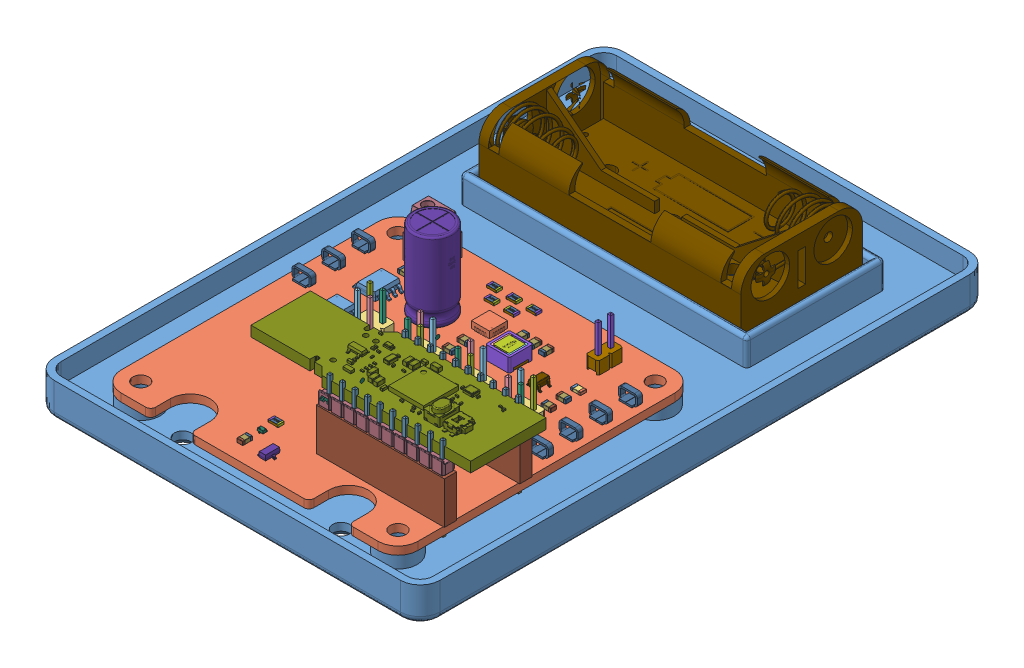
SolidWorks assembly 2228_Emetteur_Assembly, configuration Défaut. Lengths in mm.
Overall size (78 27.62 115.1).
221 component instances, 55 part files, 8 mates.
Components (placement in the parent):
- 2228_Emetteur_Bottom_wPCB-1: 2228_Emetteur_Bottom_wPCB [Défaut] at origin size (78 8.5 115.1)
- 2228_Emetteur_Top-1: 2228_Emetteur_Top [Défaut] at (0 31 0) x (-1 0 0) z (0 0 1) size (78 28 115.1) (hidden)
- 22280A_AlarmeFenetre_Emetteur.step-1: 22280A_AlarmeFenetre_Emetteur.step [Défaut] at (30 7.1063 -64.5) x (-1 0 0) z (0 1 0) size (64.32 60 20.1)
  - Board.step-1: Board.step [Défaut] at origin size (60 60 1.61)
    - Open CASCADE STEP translator 6.8 1.1.1.step-1: Open CASCADE STEP translator 6.8 1.1.1.step [Défaut] at (0 0 -1.6063) size (60 60 1.61)
  - X3.step-1: X3.step [Défaut] at origin size (5.08 5.08 11.54)
    - 61300421121.step-1: 61300421121.step [Défaut] at (31.75 25 1.27) x (0 1 0) z (1 0 0) size (5.08 11.54 5.08)
      - Open CASCADE STEP translator 6.8 1.2.1.1.step-1: Open CASCADE STEP translator 6.8 1.2.1.1.step [Défaut] at origin size (5.08 2.54 5.08)
      - Open CASCADE STEP translator 6.8 1.2.1.2.step-1: Open CASCADE STEP translator 6.8 1.2.1.2.step [Défaut] at origin size (0.64 11.54 0.64)
      - Open CASCADE STEP translator 6.8 1.2.1.3.step-1: Open CASCADE STEP translator 6.8 1.2.1.3.step [Défaut] at origin size (0.64 11.54 0.64)
      - Open CASCADE STEP translator 6.8 1.2.1.4.step-1: Open CASCADE STEP translator 6.8 1.2.1.4.step [Défaut] at origin size (0.64 11.54 0.64)
      - Open CASCADE STEP translator 6.8 1.2.1.5.step-1: Open CASCADE STEP translator 6.8 1.2.1.5.step [Défaut] at origin size (0.64 11.54 0.64)
  - X5.step-1: X5.step [Défaut] at origin size (5.08 5.08 11.54)
    - 61300421121.step-1: 61300421121.step [Défaut] at (21.59 25 1.27) x (0 1 0) z (1 0 0) size (5.08 11.54 5.08)
      - Open CASCADE STEP translator 6.8 1.2.1.1.step-1: Open CASCADE STEP translator 6.8 1.2.1.1.step [Défaut] at origin size (5.08 2.54 5.08)
      - Open CASCADE STEP translator 6.8 1.2.1.2.step-1: Open CASCADE STEP translator 6.8 1.2.1.2.step [Défaut] at origin size (0.64 11.54 0.64)
      - Open CASCADE STEP translator 6.8 1.2.1.3.step-1: Open CASCADE STEP translator 6.8 1.2.1.3.step [Défaut] at origin size (0.64 11.54 0.64)
      - Open CASCADE STEP translator 6.8 1.2.1.4.step-1: Open CASCADE STEP translator 6.8 1.2.1.4.step [Défaut] at origin size (0.64 11.54 0.64)
      - Open CASCADE STEP translator 6.8 1.2.1.5.step-1: Open CASCADE STEP translator 6.8 1.2.1.5.step [Défaut] at origin size (0.64 11.54 0.64)
  - X4.step-1: X4.step [Défaut] at origin size (5.08 5.08 11.54)
    - 61300421121.step-1: 61300421121.step [Défaut] at (10.16 26.27 1.27) x (-1 0 0) z (0 1 0) size (5.08 11.54 5.08)
      - Open CASCADE STEP translator 6.8 1.2.1.1.step-1: Open CASCADE STEP translator 6.8 1.2.1.1.step [Défaut] at origin size (5.08 2.54 5.08)
      - Open CASCADE STEP translator 6.8 1.2.1.2.step-1: Open CASCADE STEP translator 6.8 1.2.1.2.step [Défaut] at origin size (0.64 11.54 0.64)
      - Open CASCADE STEP translator 6.8 1.2.1.3.step-1: Open CASCADE STEP translator 6.8 1.2.1.3.step [Défaut] at origin size (0.64 11.54 0.64)
      - Open CASCADE STEP translator 6.8 1.2.1.4.step-1: Open CASCADE STEP translator 6.8 1.2.1.4.step [Défaut] at origin size (0.64 11.54 0.64)
      - Open CASCADE STEP translator 6.8 1.2.1.5.step-1: Open CASCADE STEP translator 6.8 1.2.1.5.step [Défaut] at origin size (0.64 11.54 0.64)
  - X2.step-1: X2.step [Défaut] at origin size (5.08 5.08 11.54)
    - 61300421121.step-1: 61300421121.step [Défaut] at (39.37 25 1.27) x (0 -1 0) z (-1 0 0) size (5.08 11.54 5.08)
      - Open CASCADE STEP translator 6.8 1.2.1.1.step-1: Open CASCADE STEP translator 6.8 1.2.1.1.step [Défaut] at origin size (5.08 2.54 5.08)
      - Open CASCADE STEP translator 6.8 1.2.1.2.step-1: Open CASCADE STEP translator 6.8 1.2.1.2.step [Défaut] at origin size (0.64 11.54 0.64)
      - Open CASCADE STEP translator 6.8 1.2.1.3.step-1: Open CASCADE STEP translator 6.8 1.2.1.3.step [Défaut] at origin size (0.64 11.54 0.64)
      - Open CASCADE STEP translator 6.8 1.2.1.4.step-1: Open CASCADE STEP translator 6.8 1.2.1.4.step [Défaut] at origin size (0.64 11.54 0.64)
      - Open CASCADE STEP translator 6.8 1.2.1.5.step-1: Open CASCADE STEP translator 6.8 1.2.1.5.step [Défaut] at origin size (0.64 11.54 0.64)
  - X1.step-1: X1.step [Défaut] at origin size (2.54 5.08 11.54)
    - STEP-61300211121-rev1.step-1: STEP-61300211121-rev1.step [Défaut] at (11.9999 6.27 1.27) x (0 -1 0) z (-1 0 0) size (5.08 11.54 2.54)
      - 6130xx11121_PIN.step-1: 6130xx11121_PIN.step [Défaut] at (-1.27 1.5 0) x (1 0 0) z (0 -1 0) size (0.64 0.64 11.54)
      - 6130xx11121_PIN.step-2: 6130xx11121_PIN.step [Défaut] at (1.27 1.5 0) x (1 0 0) z (0 -1 0) size (0.64 0.64 11.54)
      - 61300211121.step-1: 61300211121.step [Défaut] at origin size (5.08 2.54 2.54)
  - VSTOR.step-1: VSTOR.step [Défaut] at origin size (3.81 2.03 2.29)
    - keystone-PN5019.step-1: keystone-PN5019.step [Défaut] at (56.9999 22.0009 0) x (1 0 0) z (0 -1 0) size (3.81 2.29 2.03)
  - VSEC.step-1: VSEC.step [Défaut] at origin size (3.81 2.03 2.29)
    - keystone-PN5019.step-1: keystone-PN5019.step [Défaut] at (57.0001 15.9991 0) x (-1 0 0) z (0 1 0) size (3.81 2.29 2.03)
  - VMUL.step-1: VMUL.step [Défaut] at origin size (3.81 2.03 2.29)
    - keystone-PN5019.step-1: keystone-PN5019.step [Défaut] at (3.0001 21.9991 0) x (-1 0 0) z (0 1 0) size (3.81 2.29 2.03)
  - VIN.step-1: VIN.step [Défaut] at origin size (3.81 2.03 2.29)
    - keystone-PN5019.step-1: keystone-PN5019.step [Défaut] at (2.9999 10.0009 0) x (1 0 0) z (0 -1 0) size (3.81 2.29 2.03)
  - VCC.step-1: VCC.step [Défaut] at origin size (3.81 2.03 2.29)
    - keystone-PN5019.step-1: keystone-PN5019.step [Défaut] at (3.0001 27.9991 0) x (-1 0 0) z (0 1 0) size (3.81 2.29 2.03)
  - U6.step-1: U6.step [Défaut] at origin size (46.04 19.26 18.6)
    - 61301011821.step-1: 61301011821.step [Défaut] at (1.27 49.62 0) x (1 0 0) z (0 0 1) size (25.9 2.5 11.6)
      - Body.step-1: Body.step [Défaut] at origin size (25.9 2.5 8.5)
      - LeadsArray.step-1: LeadsArray.step [Défaut] at origin size (23.46 0.6 4.8)
    - 61301011821.step-2: 61301011821.step [Défaut] at (1.27 34.38 0) x (1 0 0) z (0 0 1) size (25.9 2.5 11.6)
      - Body.step-1: Body.step [Défaut] at origin size (25.9 2.5 8.5)
      - LeadsArray.step-1: LeadsArray.step [Défaut] at origin size (23.46 0.6 4.8)
    - Conn_Wurth_Elektronik_61301011121_eec.step-1: Conn_Wurth_Elektronik_61301011121_eec.step [Défaut] at (12.7 49.62 10) x (1 0 0) z (0 1 0) size (25.4 11.74 4.02)
      - Package.step-1: Package.step [Défaut] at origin size (25.4 2.54 2.54)
      - Pins.step-1: Pins.step [Défaut] at origin size (23.5 11.74 0.64)
      - Logo.step-1: Logo.step [Défaut] at (12.7 -1.27 1.27) size (5.18 4.49 4.02)
    - Conn_Wurth_Elektronik_61301011121_eec.step-2: Conn_Wurth_Elektronik_61301011121_eec.step [Défaut] at (12.7 34.38 10) x (1 0 0) z (0 1 0) size (25.4 11.74 4.02)
      - Package.step-1: Package.step [Défaut] at origin size (25.4 2.54 2.54)
      - Pins.step-1: Pins.step [Défaut] at origin size (23.5 11.74 0.64)
      - Logo.step-1: Logo.step [Défaut] at (12.7 -1.27 1.27) size (5.18 4.49 4.02)
    - 400250.step-1: 400250.step [Défaut] at (-4.318 42 13) x (1 0 0) z (0 0 1) size (46.04 15.24 4.57)
  - U5.step-1: U5.step [Défaut] at origin size (2.51 2.92 1.12)
    - 5881998176.step-1: 5881998176.step [Défaut] at (30 56 0) x (-1 0 0) z (0 1 0) size (2.51 1.12 2.92)
  - U4.step-1: U4.step [Défaut] at origin size (2.8 2.9 1.45)
    - 5881997696.step-1: 5881997696.step [Défaut] at (15 16.5 0) x (-1 0 0) z (0 1 0) size (2.8 1.45 2.9)
  - U3.step-1: U3.step [Défaut] at origin size (6.1 4.99 1.77)
    - 5882000496.step-1: 5882000496.step [Défaut] at (48 16 0) x (-1 0 0) z (0 0 1) size (6.1 4.99 1.77)
  - U2.step-1: U2.step [Défaut] at origin size (6.1 4.99 1.77)
    - 5882000496.step-1: 5882000496.step [Défaut] at (48 25 0) x (-1 0 0) z (0 0 1) size (6.1 4.99 1.77)
  - U1.step-1: U1.step [Défaut] at origin size (3.76 3.76 1.4)
    - RGR20_2P05X2P05_TEX.step-1: RGR20_2P05X2P05_TEX.step [Défaut] at (30 11.5 0) x (1 0 0) z (0 0 1) size (3.76 3.76 1.4)
  - S1.step-1: S1.step [Défaut] at origin size (23 8 1.9)
    - Anysolar_KXOB25.step-1: Anysolar_KXOB25.step [Défaut] at (30 5 -1.6063) x (1 0 0) z (0 0 -1) size (7.2 6.59 0.1)
    - Anysolar_KXOB25-0.step-1: Anysolar_KXOB25-0.step [Défaut] at (30 5 -1.6063) x (1 0 0) z (0 0 -1) size (23 8 1.8)
    - Anysolar_KXOB25-1.step-1: Anysolar_KXOB25-1.step [Défaut] at (30 5 -1.6063) x (1 0 0) z (0 0 -1) size (7.2 6.59 0.1)
    - Anysolar_KXOB25-2.step-1: Anysolar_KXOB25-2.step [Défaut] at (30 5 -1.6063) x (1 0 0) z (0 0 -1) size (7.2 6.59 0.1)
  - R6.step-1: R6.step [Défaut] at origin size (2 1.25 0.51)
    - Resistor_0805_Text.step-1: Resistor_0805_Text.step [Défaut] at (35 49.62 0) x (1 0 0) z (0 0 1) size (2 1.25 0.51)
      - Pin1Body.step-1: Pin1Body.step [Défaut] at (0 0 0.01) size (0.37 1.25 0.5)
      - Pin2Body.step-1: Pin2Body.step [Défaut] at (0 0 0.01) size (0.37 1.25 0.5)
      - CeramicBody.step-1: CeramicBody.step [Défaut] at (0 0 0.01) size (1.93 1.25 0.43)
      - CoatingBody.step-1: CoatingBody.step [Défaut] at (0 0 0.01) size (1.33 1.25 0.03)
      - Text1Body.step-1: Text1Body.step [Défaut] at (0 0 0.01) size (0.25 0.4 0.01)
      - Text2Body.step-1: Text2Body.step [Défaut] at (0 0 0.01) size (0.25 0.4 0.01)
      - Text3Body.step-1: Text3Body.step [Défaut] at (0 0 0.01) size (0.25 0.4 0.01)
      - Text4Body.step-1: Text4Body.step [Défaut] at (0 0 0.01) size (0.25 0.4 0.01)
  - R5.step-1: R5.step [Défaut] at origin size (2 1.25 0.51)
    - Resistor_0805_Text.step-1: Resistor_0805_Text.step [Défaut] at (32.5 4 0) x (1 0 0) z (0 0 1) size (2 1.25 0.51)
      - Pin1Body.step-1: Pin1Body.step [Défaut] at (0 0 0.01) size (0.37 1.25 0.5)
      - Pin2Body.step-1: Pin2Body.step [Défaut] at (0 0 0.01) size (0.37 1.25 0.5)
      - CeramicBody.step-1: CeramicBody.step [Défaut] at (0 0 0.01) size (1.93 1.25 0.43)
      - CoatingBody.step-1: CoatingBody.step [Défaut] at (0 0 0.01) size (1.33 1.25 0.03)
      - Text1Body.step-1: Text1Body.step [Défaut] at (0 0 0.01) size (0.25 0.4 0.01)
      - Text2Body.step-1: Text2Body.step [Défaut] at (0 0 0.01) size (0.25 0.4 0.01)
      - Text3Body.step-1: Text3Body.step [Défaut] at (0 0 0.01) size (0.25 0.4 0.01)
      - Text4Body.step-1: Text4Body.step [Défaut] at (0 0 0.01) size (0.25 0.4 0.01)
  - R4.step-1: R4.step [Défaut] at origin size (2 1.25 0.51)
    - Resistor_0805_Text.step-1: Resistor_0805_Text.step [Défaut] at (34.5 6.5 0) x (1 0 0) z (0 0 1) size (2 1.25 0.51)
      - Pin1Body.step-1: Pin1Body.step [Défaut] at (0 0 0.01) size (0.37 1.25 0.5)
      - Pin2Body.step-1: Pin2Body.step [Défaut] at (0 0 0.01) size (0.37 1.25 0.5)
      - CeramicBody.step-1: CeramicBody.step [Défaut] at (0 0 0.01) size (1.93 1.25 0.43)
      - CoatingBody.step-1: CoatingBody.step [Défaut] at (0 0 0.01) size (1.33 1.25 0.03)
      - Text1Body.step-1: Text1Body.step [Défaut] at (0 0 0.01) size (0.25 0.4 0.01)
      - Text2Body.step-1: Text2Body.step [Défaut] at (0 0 0.01) size (0.25 0.4 0.01)
      - Text3Body.step-1: Text3Body.step [Défaut] at (0 0 0.01) size (0.25 0.4 0.01)
      - Text4Body.step-1: Text4Body.step [Défaut] at (0 0 0.01) size (0.25 0.4 0.01)
  - R3.step-1: R3.step [Défaut] at origin size (2 1.25 0.51)
    - Resistor_0805_Text.step-1: Resistor_0805_Text.step [Défaut] at (36.5 4 0) x (1 0 0) z (0 0 1) size (2 1.25 0.51)
      - Pin1Body.step-1: Pin1Body.step [Défaut] at (0 0 0.01) size (0.37 1.25 0.5)
      - Pin2Body.step-1: Pin2Body.step [Défaut] at (0 0 0.01) size (0.37 1.25 0.5)
      - CeramicBody.step-1: CeramicBody.step [Défaut] at (0 0 0.01) size (1.93 1.25 0.43)
      - CoatingBody.step-1: CoatingBody.step [Défaut] at (0 0 0.01) size (1.33 1.25 0.03)
      - Text1Body.step-1: Text1Body.step [Défaut] at (0 0 0.01) size (0.25 0.4 0.01)
      - Text2Body.step-1: Text2Body.step [Défaut] at (0 0 0.01) size (0.25 0.4 0.01)
      - Text3Body.step-1: Text3Body.step [Défaut] at (0 0 0.01) size (0.25 0.4 0.01)
      - Text4Body.step-1: Text4Body.step [Défaut] at (0 0 0.01) size (0.25 0.4 0.01)
  - R2.step-1: R2.step [Défaut] at origin size (2 1.25 0.51)
    - Resistor_0805_Text.step-1: Resistor_0805_Text.step [Défaut] at (30.5 6.5 0) x (-1 0 0) z (0 0 1) size (2 1.25 0.51)
      - Pin1Body.step-1: Pin1Body.step [Défaut] at (0 0 0.01) size (0.37 1.25 0.5)
      - Pin2Body.step-1: Pin2Body.step [Défaut] at (0 0 0.01) size (0.37 1.25 0.5)
      - CeramicBody.step-1: CeramicBody.step [Défaut] at (0 0 0.01) size (1.93 1.25 0.43)
      - CoatingBody.step-1: CoatingBody.step [Défaut] at (0 0 0.01) size (1.33 1.25 0.03)
      - Text1Body.step-1: Text1Body.step [Défaut] at (0 0 0.01) size (0.25 0.4 0.01)
      - Text2Body.step-1: Text2Body.step [Défaut] at (0 0 0.01) size (0.25 0.4 0.01)
      - Text3Body.step-1: Text3Body.step [Défaut] at (0 0 0.01) size (0.25 0.4 0.01)
      - Text4Body.step-1: Text4Body.step [Défaut] at (0 0 0.01) size (0.25 0.4 0.01)
  - R1.step-1: R1.step [Défaut] at origin size (2 1.25 0.51)
    - Resistor_0805_Text.step-1: Resistor_0805_Text.step [Défaut] at (28.5 4 0) x (-1 0 0) z (0 0 1) size (2 1.25 0.51)
      - Pin1Body.step-1: Pin1Body.step [Défaut] at (0 0 0.01) size (0.37 1.25 0.5)
      - Pin2Body.step-1: Pin2Body.step [Défaut] at (0 0 0.01) size (0.37 1.25 0.5)
      - CeramicBody.step-1: CeramicBody.step [Défaut] at (0 0 0.01) size (1.93 1.25 0.43)
      - CoatingBody.step-1: CoatingBody.step [Défaut] at (0 0 0.01) size (1.33 1.25 0.03)
      - Text1Body.step-1: Text1Body.step [Défaut] at (0 0 0.01) size (0.25 0.4 0.01)
      - Text2Body.step-1: Text2Body.step [Défaut] at (0 0 0.01) size (0.25 0.4 0.01)
      - Text3Body.step-1: Text3Body.step [Défaut] at (0 0 0.01) size (0.25 0.4 0.01)
      - Text4Body.step-1: Text4Body.step [Défaut] at (0 0 0.01) size (0.25 0.4 0.01)
  - Q1.step-1: Q1.step [Défaut] at origin size (1.2 1.2 0.55)
    - Trans_Rohm_RZM001P02T2L_eec.step-1: Trans_Rohm_RZM001P02T2L_eec.step [Défaut] at (35 52.5 0) x (0 1 0) z (0 0 1) size (1.2 1.2 0.55)
      - 1.step-1: 1.step [Défaut] at (0 0 0.05) x (0 -1 0) z (0 0 1) size (1.2 0.8 0.5)
      - 2.step-1: 2.step [Défaut] x (0 -1 0) z (0 0 1) size (1.02 1.2 0.13)
      - 3.step-1: 3.step [Défaut] at (0.0085 -0.0135 0.451) x (0 -1 0) z (0 0 1) size (0.31 0.18 0.11)
      - Notch.step-1: Notch.step [Défaut] at (-4.7119 3.8027 0.451) size (0.08 0.08 0.1)
  - L2.step-1: L2.step [Défaut] at origin size (2 1.25 0.6)
    - L_0805.step-1: L_0805.step [Défaut] at (10 13.5 0) x (-1 0 0) z (0 0 1) size (2 1.25 0.6)
      - Pin1.step-1: Pin1.step [Défaut] at origin size (0.62 1.25 0.6)
      - Pin2.step-1: Pin2.step [Défaut] at origin size (0.62 1.25 0.6)
      - CeramicBody-3.step-1: CeramicBody-3.step [Défaut] at origin size (1.8 1.23 0.58)
  - L1.step-1: L1.step [Défaut] at origin size (4.8 4.8 2.8)
    - 4828_74406043.step-1: 4828_74406043.step [Défaut] at (22.0529 15.7176 0) x (1 0 0) z (0 0 1) size (4.8 4.8 2.8)
      - Glue_L.step-1: Glue_L.step [Défaut] at (2.097 -0.9177 0.85) x (0 1 0) z (0 0 1) size (3.9 0.6 1.97)
      - Glue_R.step-1: Glue_R.step [Défaut] at (-1.203 -0.5177 0.85) x (0 1 0) z (0 0 1) size (3.9 0.6 1.95)
      - 4828_74406043-4.step-1: 4828_74406043-4.step [Défaut] at (0.447 -2.3677 0.001) size (3.26 2.73 2.5)
      - 4828_74406043-5.step-1: 4828_74406043-5.step [Défaut] at (0.447 -2.3677 0.001) size (3.9 3.3 2.8)
      - 4828_74406043_Housing.step-1: 4828_74406043_Housing.step [Défaut] at (0.447 -0.7177 0) size (4.8 4.8 2.8)
      - 4828_74406043_Pads.step-1: 4828_74406043_Pads.step [Défaut] at (-1.153 -0.7177 0) size (1.6 3.3 0.6)
      - 4828_74406043_Pads.step-2: 4828_74406043_Pads.step [Défaut] at (2.047 -0.7177 0) x (-1 0 0) z (0 0 1) size (1.6 3.3 0.6)
  - GND2.step-1: GND2.step [Défaut] at origin size (3.81 2.03 2.29)
    - keystone-PN5019.step-1: keystone-PN5019.step [Défaut] at (57.0001 9.9991 0) x (-1 0 0) z (0 1 0) size (3.81 2.29 2.03)
  - GND1.step-1: GND1.step [Défaut] at origin size (3.81 2.03 2.29)
    - keystone-PN5019.step-1: keystone-PN5019.step [Défaut] at (3.0001 15.9991 0) x (-1 0 0) z (0 1 0) size (3.81 2.29 2.03)
  - C9.step-1: C9.step [Défaut] at origin size (1.25 2 0.8)
    - Ceramic_Capacitor_0805_h32mil.step-1: Ceramic_Capacitor_0805_h32mil.step [Défaut] at (35 56 0) x (0 1 0) z (0 0 1) size (2 1.25 0.8)
      - Pin1-6.step-1: Pin1-6.step [Défaut] at origin size (0.62 1.25 0.8)
      - Pin2-7.step-1: Pin2-7.step [Défaut] at origin size (0.62 1.25 0.8)
      - CeramicBody-8.step-1: CeramicBody-8.step [Défaut] at origin size (1.8 1.23 0.78)
  - C8.step-1: C8.step [Défaut] at origin size (2 1.25 0.8)
    - Ceramic_Capacitor_0805_h32mil.step-1: Ceramic_Capacitor_0805_h32mil.step [Défaut] at (10 19.5 0) x (-1 0 0) z (0 0 1) size (2 1.25 0.8)
      - Pin1-6.step-1: Pin1-6.step [Défaut] at origin size (0.62 1.25 0.8)
      - Pin2-7.step-1: Pin2-7.step [Défaut] at origin size (0.62 1.25 0.8)
      - CeramicBody-8.step-1: CeramicBody-8.step [Défaut] at origin size (1.8 1.23 0.78)
  - C7.step-1: C7.step [Défaut] at origin size (2 1.25 0.8)
    - Ceramic_Capacitor_0805_h32mil.step-1: Ceramic_Capacitor_0805_h32mil.step [Défaut] at (10 16.5 0) x (1 0 0) z (0 0 1) size (2 1.25 0.8)
      - Pin1-6.step-1: Pin1-6.step [Défaut] at origin size (0.62 1.25 0.8)
      - Pin2-7.step-1: Pin2-7.step [Défaut] at origin size (0.62 1.25 0.8)
      - CeramicBody-8.step-1: CeramicBody-8.step [Défaut] at origin size (1.8 1.23 0.78)
  - C6.step-1: C6.step [Défaut] at origin size (2 1.25 0.8)
    - Ceramic_Capacitor_0805_h32mil.step-1: Ceramic_Capacitor_0805_h32mil.step [Défaut] at (30 16.5 0) x (1 0 0) z (0 0 1) size (2 1.25 0.8)
      - Pin1-6.step-1: Pin1-6.step [Défaut] at origin size (0.62 1.25 0.8)
      - Pin2-7.step-1: Pin2-7.step [Défaut] at origin size (0.62 1.25 0.8)
      - CeramicBody-8.step-1: CeramicBody-8.step [Défaut] at origin size (1.8 1.23 0.78)
  - C5.step-1: C5.step [Défaut] at origin size (2 1.25 0.8)
    - Ceramic_Capacitor_0805_h32mil.step-1: Ceramic_Capacitor_0805_h32mil.step [Défaut] at (30 19.5 0) x (1 0 0) z (0 0 1) size (2 1.25 0.8)
      - Pin1-6.step-1: Pin1-6.step [Défaut] at origin size (0.62 1.25 0.8)
      - Pin2-7.step-1: Pin2-7.step [Défaut] at origin size (0.62 1.25 0.8)
      - CeramicBody-8.step-1: CeramicBody-8.step [Défaut] at origin size (1.8 1.23 0.78)
  - C4.step-1: C4.step [Défaut] at origin size (2 1.25 0.8)
    - Ceramic_Capacitor_0805_h32mil.step-1: Ceramic_Capacitor_0805_h32mil.step [Défaut] at (48 10.5 0) x (-1 0 0) z (0 0 1) size (2 1.25 0.8)
      - Pin1-6.step-1: Pin1-6.step [Défaut] at origin size (0.62 1.25 0.8)
      - Pin2-7.step-1: Pin2-7.step [Défaut] at origin size (0.62 1.25 0.8)
      - CeramicBody-8.step-1: CeramicBody-8.step [Défaut] at origin size (1.8 1.23 0.78)
  - C3.step-1: C3.step [Défaut] at origin size (1.25 2 0.8)
    - Ceramic_Capacitor_0805_h32mil.step-1: Ceramic_Capacitor_0805_h32mil.step [Défaut] at (25 10 0) x (0 1 0) z (0 0 1) size (2 1.25 0.8)
      - Pin1-6.step-1: Pin1-6.step [Défaut] at origin size (0.62 1.25 0.8)
      - Pin2-7.step-1: Pin2-7.step [Défaut] at origin size (0.62 1.25 0.8)
      - CeramicBody-8.step-1: CeramicBody-8.step [Défaut] at origin size (1.8 1.23 0.78)
  - C2.step-1: C2.step [Défaut] at origin size (1.25 2 0.8)
    - Ceramic_Capacitor_0805_h32mil.step-1: Ceramic_Capacitor_0805_h32mil.step [Défaut] at (22.5 10 0) x (0 -1 0) z (0 0 1) size (2 1.25 0.8)
      - Pin1-6.step-1: Pin1-6.step [Défaut] at origin size (0.62 1.25 0.8)
      - Pin2-7.step-1: Pin2-7.step [Défaut] at origin size (0.62 1.25 0.8)
      - CeramicBody-8.step-1: CeramicBody-8.step [Défaut] at origin size (1.8 1.23 0.78)
  - C1.step-1: C1.step [Défaut] at origin size (1.25 2 0.8)
    - Ceramic_Capacitor_0805_h32mil.step-1: Ceramic_Capacitor_0805_h32mil.step [Défaut] at (20 10 0) x (0 -1 0) z (0 0 1) size (2 1.25 0.8)
      - Pin1-6.step-1: Pin1-6.step [Défaut] at origin size (0.62 1.25 0.8)
      - Pin2-7.step-1: Pin2-7.step [Défaut] at origin size (0.62 1.25 0.8)
      - CeramicBody-8.step-1: CeramicBody-8.step [Défaut] at origin size (1.8 1.23 0.78)
  - B2.step-1: B2.step [Défaut] at origin size (5.48 6.84 12.4)
    - Conn_W_rth_Elektronik_691210910002_eec.step-1: Conn_W_rth_Elektronik_691210910002_eec.step [Défaut] at (48 5 0) size (5.48 6.84 12.4)
      - 691210910002.step-1: 691210910002.step [Défaut] at (0 0 2.45) size (5.48 6.5 8.7)
      - 6912109100xx_CAGE.step-1: 6912109100xx_CAGE.step [Défaut] at (1.27 -0.175 2.65) size (2 3 3.9)
      - 6912109100xx_PIN.step-1: 6912109100xx_PIN.step [Défaut] at (1.27 0.195 1.8) x (-1 0 0) z (0 1 0) size (2.15 7.1 3.9)
      - 6912109100xx_VIS.step-1: 6912109100xx_VIS.step [Défaut] at (-1.27 -0.25 3.3) x (0 -1 0) z (0 0 1) size (2.1 2.1 4.45)
      - 6912109100xx_PIN.step-2: 6912109100xx_PIN.step [Défaut] at (-1.27 0.195 1.8) x (-1 0 0) z (0 1 0) size (2.15 7.1 3.9)
      - 6912109100xx_CAGE.step-2: 6912109100xx_CAGE.step [Défaut] at (-1.27 -0.175 2.65) size (2 3 3.9)
      - 6912109100xx_VIS.step-2: 6912109100xx_VIS.step [Défaut] at (1.27 -0.25 3.3) x (0 -1 0) z (0 0 1) size (2.1 2.1 4.45)
      - Logo.step-1: Logo.step [Défaut] at (2.74 -2.9 4.5) x (1 0 0) z (0 -0.972937 0.231072) size (5.18 4.49 4.02)
  - B1.step-1: B1.step [Défaut] at origin size (8.38 8 20.1)
    - 220uF_35V_electr_8_x16mm_-P.diameter_4mm.step-1: 220uF_35V_electr_8_x16mm_-P.diameter_4mm.step [Défaut] at (38.5 14.5 0) x (1 0 0) z (0 -1 0) size (8.38 20.1 8)
- keystone-PN2469.step-1: keystone-PN2469.step [Défaut] at (6.2774 15.2919 -91.2766) x (-1 0 0.000133) z (-0.000133 0 -1) size (69.29 27.34 37.92)
Mates (geometry in assembly coordinates):
- Coïncidente1: coincident anti-aligned: plane of 2228_Emetteur_Bottom_wPCB-1 through (0 7.05 0) normal (0 1 0); plane of 2228_Emetteur_Top-1 through (0 7.05 -57.55) normal (0 -1 0)
- Coïncidente2: coincident anti-aligned: line of 2228_Emetteur_Bottom_wPCB-1 through (-35 7.05 0) axis (1 0 0); line of 2228_Emetteur_Top-1 through (35 7.05 0) axis (-1 0 0)
- Coïncidente3: coincident anti-aligned: line of 2228_Emetteur_Bottom_wPCB-1 through (-39 7.05 -111.1) axis (0 0 1); line of 2228_Emetteur_Top-1 through (-39 7.05 -4) axis (0 0 -1)
- Coaxiale9: concentric anti-aligned: circle of 2228_Emetteur_Bottom_wPCB-1; circle of 22280A_AlarmeFenetre_Emetteur.step-1/Board.step-1/Open CASCADE STEP translator 6.8 1.1.1.step-1
- Coaxiale10: concentric aligned: cylinder of 2228_Emetteur_Bottom_wPCB-1 through (-26 1.5 -60.5) axis (0 1 0) radius 2; circle of 22280A_AlarmeFenetre_Emetteur.step-1/Board.step-1/Open CASCADE STEP translator 6.8 1.1.1.step-1
- Coïncidente6: coincident anti-aligned: plane of 2228_Emetteur_Bottom_wPCB-1 through (-26 5.5 -60.5) normal (0 1 0); plane of 22280A_AlarmeFenetre_Emetteur.step-1/Board.step-1/Open CASCADE STEP translator 6.8 1.1.1.step-1 through (26 5.5 -64.5) normal (0 -1 0)
- Coïncidente7: coincident anti-aligned: plane of 2228_Emetteur_Bottom_wPCB-1 through (0 5.5 0) normal (0 1 0); plane of keystone-PN2469.step-1 through (-26.8688 5.5 -102.2901) normal (0 -1 0)
- Coaxiale11: concentric anti-aligned: circle of 2228_Emetteur_Bottom_wPCB-1; cylinder of keystone-PN2469.step-1 through (-0.375 7.532 -90) axis (0 -1 0) radius 1.4986
